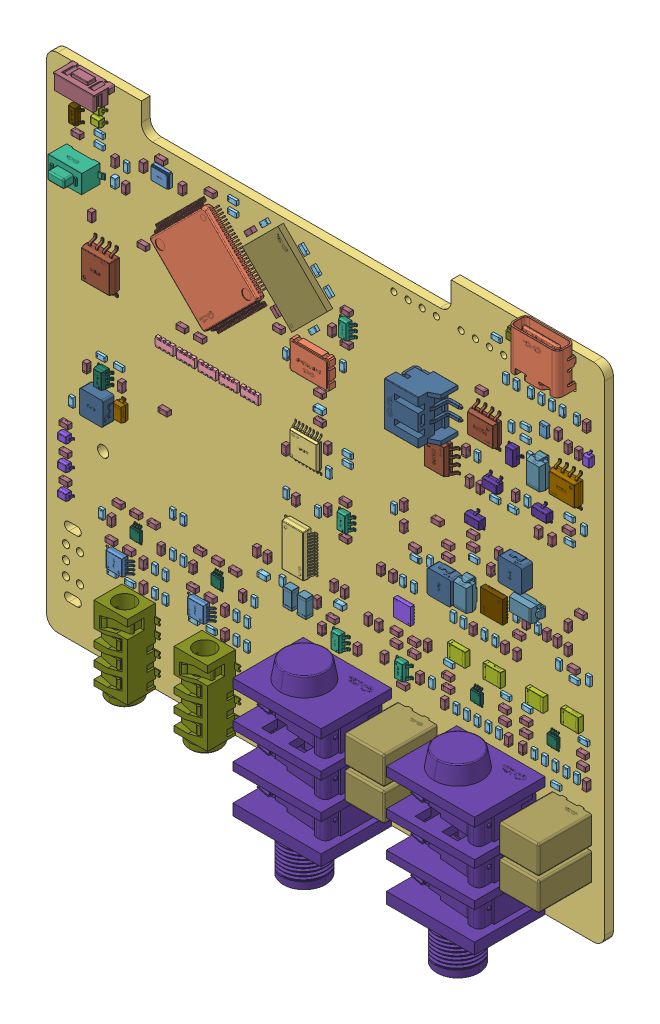
SolidWorks assembly 3D_board_2024-11-06, configuration 默认. Lengths in mm.
Overall size (99.97 100.01 16.2).
845 component instances, 39 part files, 0 mates.
Components (placement in the parent):
- 3D_board_2024-11-06.step-1: 3D_board_2024-11-06.step [默认] at origin size (99.97 100.01 16.2)
  - iqks-X1.step-1: iqks-X1.step [默认] at (20.955 -9.525 1.5862) x (-1 0 0) z (0 0 1) size (3.2 2.5 0.81)
    - OSC-SMD_4P-L3.2-W2.5-BL.step-1: OSC-SMD_4P-L3.2-W2.5-BL.step [默认] at origin size (3.2 2.5 0.81)
      - SOLID.step-1: SOLID.step [默认] at origin size (3.2 2.5 0.81)
  - iqks-X2.step-1: iqks-X2.step [默认] at (48.2601 -24.765 1.5862) x (-1 0 0) z (0 0 1) size (7 5 1.32)
    - OSC-SMD_4P-L7.0-W5.0-BL.step-1: OSC-SMD_4P-L7.0-W5.0-BL.step [默认] at origin size (7 5 1.32)
      - COMPOUND.step-1: COMPOUND.step [默认] at origin size (7 5 1.32)
  - iqks-U22.step-1: iqks-U22.step [默认] at (45.7201 -54.6101 1.5862) x (-1 0 0) z (0 0 1) size (5.89 7.71 1.66)
    - SSOP-28_L10.2-W5.3-P0.65-LS7.8-BL.step-1: SSOP-28_L10.2-W5.3-P0.65-LS7.8-BL.step [默认] at origin size (5.89 7.71 1.66)
      - SOLID-0.step-1: SOLID-0.step [默认] at origin size (5.89 7.71 1.66)
  - iqks-RN4.step-1: iqks-RN4.step [默认] at (33.0201 -35.5601 1.5862) x (-1 0 0) z (0 0 1) size (3.2 1.6 0.5)
    - RES-ARRAY-SMD_0603-8P-L3.2-W1.6-BL.step-1: RES-ARRAY-SMD_0603-8P-L3.2-W1.6-BL.step [默认] at origin size (3.2 1.6 0.5)
      - COMPOUND-1.step-1: COMPOUND-1.step [默认] at origin size (3.2 1.6 0.5)
  - iqks-RN3.step-1: iqks-RN3.step [默认] at (29.2101 -35.5601 1.5862) x (-1 0 0) z (0 0 1) size (3.2 1.6 0.5)
    - RES-ARRAY-SMD_0603-8P-L3.2-W1.6-BL.step-1: RES-ARRAY-SMD_0603-8P-L3.2-W1.6-BL.step [默认] at origin size (3.2 1.6 0.5)
      - COMPOUND-1.step-1: COMPOUND-1.step [默认] at origin size (3.2 1.6 0.5)
  - iqks-RN2.step-1: iqks-RN2.step [默认] at (25.4001 -35.5601 1.5862) x (-1 0 0) z (0 0 1) size (3.2 1.6 0.5)
    - RES-ARRAY-SMD_0603-8P-L3.2-W1.6-BL.step-1: RES-ARRAY-SMD_0603-8P-L3.2-W1.6-BL.step [默认] at origin size (3.2 1.6 0.5)
      - COMPOUND-1.step-1: COMPOUND-1.step [默认] at origin size (3.2 1.6 0.5)
  - iqks-RN1.step-1: iqks-RN1.step [默认] at (21.59 -35.5601 1.5862) x (-1 0 0) z (0 0 1) size (3.2 1.6 0.5)
    - RES-ARRAY-SMD_0603-8P-L3.2-W1.6-BL.step-1: RES-ARRAY-SMD_0603-8P-L3.2-W1.6-BL.step [默认] at origin size (3.2 1.6 0.5)
      - COMPOUND-1.step-1: COMPOUND-1.step [默认] at origin size (3.2 1.6 0.5)
  - iqks-RN5.step-1: iqks-RN5.step [默认] at (36.8301 -35.5601 1.5862) x (-1 0 0) z (0 0 1) size (3.2 1.6 0.5)
    - RES-ARRAY-SMD_0603-8P-L3.2-W1.6-BL.step-1: RES-ARRAY-SMD_0603-8P-L3.2-W1.6-BL.step [默认] at origin size (3.2 1.6 0.5)
      - COMPOUND-1.step-1: COMPOUND-1.step [默认] at origin size (3.2 1.6 0.5)
  - iqks-R53.step-1: iqks-R53.step [默认] at (90.8052 -10.16 1.5862) x (0 1 0) z (0 0 1) size (1.62 0.81 0.45)
    - R0603.step-1: R0603.step [默认] at origin size (1.62 0.81 0.45)
      - COMPOUND-2.step-1: COMPOUND-2.step [默认] at origin size (1.62 0.81 0.45)
  - iqks-R52.step-1: iqks-R52.step [默认] at (88.9002 -10.16 1.5862) x (0 1 0) z (0 0 1) size (1.62 0.81 0.45)
    - R0603.step-1: R0603.step [默认] at origin size (1.62 0.81 0.45)
      - COMPOUND-2.step-1: COMPOUND-2.step [默认] at origin size (1.62 0.81 0.45)
  - iqks-R7.step-1: iqks-R7.step [默认] at (72.3901 -59.4601 1.5862) size (1.62 0.81 0.45)
    - R0603.step-1: R0603.step [默认] at origin size (1.62 0.81 0.45)
      - COMPOUND-2.step-1: COMPOUND-2.step [默认] at origin size (1.62 0.81 0.45)
  - iqks-R14.step-1: iqks-R14.step [默认] at (82.5502 -59.4601 1.5862) x (-1 0 0) z (0 0 1) size (1.62 0.81 0.45)
    - R0603.step-1: R0603.step [默认] at origin size (1.62 0.81 0.45)
      - COMPOUND-2.step-1: COMPOUND-2.step [默认] at origin size (1.62 0.81 0.45)
  - iqks-R69.step-1: iqks-R69.step [默认] at (50.8001 -40.6401 1.5862) x (0 -1 0) z (0 0 1) size (1.62 0.81 0.45)
    - R0603.step-1: R0603.step [默认] at origin size (1.62 0.81 0.45)
      - COMPOUND-2.step-1: COMPOUND-2.step [默认] at origin size (1.62 0.81 0.45)
  - iqks-R55.step-1: iqks-R55.step [默认] at (84.4552 -10.16 1.5862) x (0 1 0) z (0 0 1) size (1.62 0.81 0.45)
    - R0603.step-1: R0603.step [默认] at origin size (1.62 0.81 0.45)
      - COMPOUND-2.step-1: COMPOUND-2.step [默认] at origin size (1.62 0.81 0.45)
  - iqks-R59.step-1: iqks-R59.step [默认] at (53.3401 -22.86 1.5862) x (0 1 0) z (0 0 1) size (1.62 0.81 0.45)
    - R0603.step-1: R0603.step [默认] at origin size (1.62 0.81 0.45)
      - COMPOUND-2.step-1: COMPOUND-2.step [默认] at origin size (1.62 0.81 0.45)
  - iqks-R62.step-1: iqks-R62.step [默认] at (48.1331 -19.8896 1.5862) x (0.707107 0.707107 0) z (0 0 1) size (1.62 0.81 0.45)
    - R0603.step-1: R0603.step [默认] at origin size (1.62 0.81 0.45)
      - COMPOUND-2.step-1: COMPOUND-2.step [默认] at origin size (1.62 0.81 0.45)
  - iqks-R63.step-1: iqks-R63.step [默认] at (50.8248 -12.6064 1.5862) x (0.707107 -0.707107 0) z (0 0 1) size (1.62 0.81 0.45)
    - R0603.step-1: R0603.step [默认] at origin size (1.62 0.81 0.45)
      - COMPOUND-2.step-1: COMPOUND-2.step [默认] at origin size (1.62 0.81 0.45)
  - iqks-R64.step-1: iqks-R64.step [默认] at (46.3551 -8.255 1.5862) x (-0.707107 0.707107 0) z (0 0 1) size (1.62 0.81 0.45)
    - R0603.step-1: R0603.step [默认] at origin size (1.62 0.81 0.45)
      - COMPOUND-2.step-1: COMPOUND-2.step [默认] at origin size (1.62 0.81 0.45)
  - iqks-R65.step-1: iqks-R65.step [默认] at (10.1012 -43.0318 1.5862) size (1.62 0.81 0.45)
    - R0603.step-1: R0603.step [默认] at origin size (1.62 0.81 0.45)
      - COMPOUND-2.step-1: COMPOUND-2.step [默认] at origin size (1.62 0.81 0.45)
  - iqks-R66.step-1: iqks-R66.step [默认] at (39.3701 -7.62 1.5862) x (0.707107 0.707107 0) z (0 0 1) size (1.62 0.81 0.45)
    - R0603.step-1: R0603.step [默认] at origin size (1.62 0.81 0.45)
      - COMPOUND-2.step-1: COMPOUND-2.step [默认] at origin size (1.62 0.81 0.45)
  - iqks-R67.step-1: iqks-R67.step [默认] at (48.5635 -10.414 1.5862) x (-0.707107 0.707107 0) z (0 0 1) size (1.62 0.81 0.45)
    - R0603.step-1: R0603.step [默认] at origin size (1.62 0.81 0.45)
      - COMPOUND-2.step-1: COMPOUND-2.step [默认] at origin size (1.62 0.81 0.45)
  - iqks-R74.step-1: iqks-R74.step [默认] at (82.5502 -10.16 1.5862) x (0 1 0) z (0 0 1) size (1.62 0.81 0.45)
    - R0603.step-1: R0603.step [默认] at origin size (1.62 0.81 0.45)
      - COMPOUND-2.step-1: COMPOUND-2.step [默认] at origin size (1.62 0.81 0.45)
  - iqks-R75.step-1: iqks-R75.step [默认] at (14.605 -11.303 1.5862) x (0 -1 0) z (0 0 1) size (1.62 0.81 0.45)
    - R0603.step-1: R0603.step [默认] at origin size (1.62 0.81 0.45)
      - COMPOUND-2.step-1: COMPOUND-2.step [默认] at origin size (1.62 0.81 0.45)
  - iqks-R76.step-1: iqks-R76.step [默认] at (33.6551 -8.89 1.5862) size (1.62 0.81 0.45)
    - R0603.step-1: R0603.step [默认] at origin size (1.62 0.81 0.45)
      - COMPOUND-2.step-1: COMPOUND-2.step [默认] at origin size (1.62 0.81 0.45)
  - iqks-R100.step-1: iqks-R100.step [默认] at (43.1801 -47.6251 1.5862) x (0 -1 0) z (0 0 1) size (1.62 0.81 0.45)
    - R0603.step-1: R0603.step [默认] at origin size (1.62 0.81 0.45)
      - COMPOUND-2.step-1: COMPOUND-2.step [默认] at origin size (1.62 0.81 0.45)
  - iqks-R103.step-1: iqks-R103.step [默认] at (54.2291 -36.0681 1.5862) x (-1 0 0) z (0 0 1) size (1.62 0.81 0.45)
    - R0603.step-1: R0603.step [默认] at origin size (1.62 0.81 0.45)
      - COMPOUND-2.step-1: COMPOUND-2.step [默认] at origin size (1.62 0.81 0.45)
  - iqks-R104.step-1: iqks-R104.step [默认] at (54.2291 -37.5921 1.5862) x (-1 0 0) z (0 0 1) size (1.62 0.81 0.45)
    - R0603.step-1: R0603.step [默认] at origin size (1.62 0.81 0.45)
      - COMPOUND-2.step-1: COMPOUND-2.step [默认] at origin size (1.62 0.81 0.45)
  - iqks-R10.step-1: iqks-R10.step [默认] at (79.3752 -65.8101 1.5862) x (0 -1 0) z (0 0 1) size (1.62 0.81 0.45)
    - R0603.step-1: R0603.step [默认] at origin size (1.62 0.81 0.45)
      - COMPOUND-2.step-1: COMPOUND-2.step [默认] at origin size (1.62 0.81 0.45)
  - iqks-R11.step-1: iqks-R11.step [默认] at (75.5652 -65.8101 1.5862) x (0 -1 0) z (0 0 1) size (1.62 0.81 0.45)
    - R0603.step-1: R0603.step [默认] at origin size (1.62 0.81 0.45)
      - COMPOUND-2.step-1: COMPOUND-2.step [默认] at origin size (1.62 0.81 0.45)
  - iqks-R29.step-1: iqks-R29.step [默认] at (93.3452 -65.8101 1.5862) x (0 -1 0) z (0 0 1) size (1.62 0.81 0.45)
    - R0603.step-1: R0603.step [默认] at origin size (1.62 0.81 0.45)
      - COMPOUND-2.step-1: COMPOUND-2.step [默认] at origin size (1.62 0.81 0.45)
  - iqks-R30.step-1: iqks-R30.step [默认] at (89.5352 -65.8101 1.5862) x (0 -1 0) z (0 0 1) size (1.62 0.81 0.45)
    - R0603.step-1: R0603.step [默认] at origin size (1.62 0.81 0.45)
      - COMPOUND-2.step-1: COMPOUND-2.step [默认] at origin size (1.62 0.81 0.45)
  - iqks-R5.step-1: iqks-R5.step [默认] at (87.6302 -65.8101 1.5862) x (0 -1 0) z (0 0 1) size (1.62 0.81 0.45)
    - R0603.step-1: R0603.step [默认] at origin size (1.62 0.81 0.45)
      - COMPOUND-2.step-1: COMPOUND-2.step [默认] at origin size (1.62 0.81 0.45)
  - iqks-R12.step-1: iqks-R12.step [默认] at (81.2802 -65.8101 1.5862) x (0 -1 0) z (0 0 1) size (1.62 0.81 0.45)
    - R0603.step-1: R0603.step [默认] at origin size (1.62 0.81 0.45)
      - COMPOUND-2.step-1: COMPOUND-2.step [默认] at origin size (1.62 0.81 0.45)
  - iqks-R13.step-1: iqks-R13.step [默认] at (73.6601 -65.8101 1.5862) x (0 -1 0) z (0 0 1) size (1.62 0.81 0.45)
    - R0603.step-1: R0603.step [默认] at origin size (1.62 0.81 0.45)
      - COMPOUND-2.step-1: COMPOUND-2.step [默认] at origin size (1.62 0.81 0.45)
  - iqks-R31.step-1: iqks-R31.step [默认] at (95.2502 -65.8101 1.5862) x (0 -1 0) z (0 0 1) size (1.62 0.81 0.45)
    - R0603.step-1: R0603.step [默认] at origin size (1.62 0.81 0.45)
      - COMPOUND-2.step-1: COMPOUND-2.step [默认] at origin size (1.62 0.81 0.45)
  - iqks-R115.step-1: iqks-R115.step [默认] at (83.8202 -29.8451 1.5862) x (-1 0 0) z (0 0 1) size (1.62 0.81 0.45)
    - R0603.step-1: R0603.step [默认] at origin size (1.62 0.81 0.45)
      - COMPOUND-2.step-1: COMPOUND-2.step [默认] at origin size (1.62 0.81 0.45)
  - iqks-R122.step-1: iqks-R122.step [默认] at (76.8352 -41.0211 1.5862) x (-1 0 0) z (0 0 1) size (1.62 0.81 0.45)
    - R0603.step-1: R0603.step [默认] at origin size (1.62 0.81 0.45)
      - COMPOUND-2.step-1: COMPOUND-2.step [默认] at origin size (1.62 0.81 0.45)
  - iqks-R91.step-1: iqks-R91.step [默认] at (42.5451 -61.5951 1.5862) x (0 -1 0) z (0 0 1) size (1.62 0.81 0.45)
    - R0603.step-1: R0603.step [默认] at origin size (1.62 0.81 0.45)
      - COMPOUND-2.step-1: COMPOUND-2.step [默认] at origin size (1.62 0.81 0.45)
  - iqks-R92.step-1: iqks-R92.step [默认] at (48.8951 -47.6251 1.5862) x (0 -1 0) z (0 0 1) size (1.62 0.81 0.45)
    - R0603.step-1: R0603.step [默认] at origin size (1.62 0.81 0.45)
      - COMPOUND-2.step-1: COMPOUND-2.step [默认] at origin size (1.62 0.81 0.45)
  - iqks-R111.step-1: iqks-R111.step [默认] at (24.765 -60.9601 1.5862) x (0 1 0) z (0 0 1) size (1.62 0.81 0.45)
    - R0603.step-1: R0603.step [默认] at origin size (1.62 0.81 0.45)
      - COMPOUND-2.step-1: COMPOUND-2.step [默认] at origin size (1.62 0.81 0.45)
  - iqks-R112.step-1: iqks-R112.step [默认] at (86.3602 -27.3051 1.5862) x (0 -1 0) z (0 0 1) size (1.62 0.81 0.45)
    - R0603.step-1: R0603.step [默认] at origin size (1.62 0.81 0.45)
      - COMPOUND-2.step-1: COMPOUND-2.step [默认] at origin size (1.62 0.81 0.45)
  - iqks-R128.step-1: iqks-R128.step [默认] at (73.1521 -51.8161 1.5862) x (0 -1 0) z (0 0 1) size (1.62 0.81 0.45)
    - R0603.step-1: R0603.step [默认] at origin size (1.62 0.81 0.45)
      - COMPOUND-2.step-1: COMPOUND-2.step [默认] at origin size (1.62 0.81 0.45)
  - iqks-R113.step-1: iqks-R113.step [默认] at (77.4702 -24.765 1.5862) x (0 1 0) z (0 0 1) size (1.62 0.81 0.45)
    - R0603.step-1: R0603.step [默认] at origin size (1.62 0.81 0.45)
      - COMPOUND-2.step-1: COMPOUND-2.step [默认] at origin size (1.62 0.81 0.45)
  - iqks-R6.step-1: iqks-R6.step [默认] at (86.3602 -59.4601 1.5862) size (1.62 0.81 0.45)
    - R0603.step-1: R0603.step [默认] at origin size (1.62 0.81 0.45)
      - COMPOUND-2.step-1: COMPOUND-2.step [默认] at origin size (1.62 0.81 0.45)
  - iqks-R32.step-1: iqks-R32.step [默认] at (96.5202 -59.4601 1.5862) x (-1 0 0) z (0 0 1) size (1.62 0.81 0.45)
    - R0603.step-1: R0603.step [默认] at origin size (1.62 0.81 0.45)
      - COMPOUND-2.step-1: COMPOUND-2.step [默认] at origin size (1.62 0.81 0.45)
  - iqks-R9.step-1: iqks-R9.step [默认] at (91.4402 -65.8101 1.5862) x (0 1 0) z (0 0 1) size (1.62 0.81 0.45)
    - R0603.step-1: R0603.step [默认] at origin size (1.62 0.81 0.45)
      - COMPOUND-2.step-1: COMPOUND-2.step [默认] at origin size (1.62 0.81 0.45)
  - iqks-R16.step-1: iqks-R16.step [默认] at (77.4702 -65.8101 1.5862) x (0 1 0) z (0 0 1) size (1.62 0.81 0.45)
    - R0603.step-1: R0603.step [默认] at origin size (1.62 0.81 0.45)
      - COMPOUND-2.step-1: COMPOUND-2.step [默认] at origin size (1.62 0.81 0.45)
  - iqks-R48.step-1: iqks-R48.step [默认] at (86.9952 -10.16 1.5862) x (0 1 0) z (0 0 1) size (1.62 0.81 0.45)
    - R0603.step-1: R0603.step [默认] at origin size (1.62 0.81 0.45)
      - COMPOUND-2.step-1: COMPOUND-2.step [默认] at origin size (1.62 0.81 0.45)
  - iqks-R50.step-1: iqks-R50.step [默认] at (92.7102 -10.16 1.5862) x (0 1 0) z (0 0 1) size (1.62 0.81 0.45)
    - R0603.step-1: R0603.step [默认] at origin size (1.62 0.81 0.45)
      - COMPOUND-2.step-1: COMPOUND-2.step [默认] at origin size (1.62 0.81 0.45)
  - iqks-R114.step-1: iqks-R114.step [默认] at (80.6452 -29.8451 1.5862) x (-1 0 0) z (0 0 1) size (1.62 0.81 0.45)
    - R0603.step-1: R0603.step [默认] at origin size (1.62 0.81 0.45)
      - COMPOUND-2.step-1: COMPOUND-2.step [默认] at origin size (1.62 0.81 0.45)
  - iqks-R21.step-1: iqks-R21.step [默认] at (19.685 -71.1201 1.5862) x (0 -1 0) z (0 0 1) size (1.62 0.81 0.45)
    - R0603.step-1: R0603.step [默认] at origin size (1.62 0.81 0.45)
      - COMPOUND-2.step-1: COMPOUND-2.step [默认] at origin size (1.62 0.81 0.45)
  - iqks-R22.step-1: iqks-R22.step [默认] at (19.685 -74.9301 1.5862) x (0 -1 0) z (0 0 1) size (1.62 0.81 0.45)
    - R0603.step-1: R0603.step [默认] at origin size (1.62 0.81 0.45)
      - COMPOUND-2.step-1: COMPOUND-2.step [默认] at origin size (1.62 0.81 0.45)
  - iqks-R25.step-1: iqks-R25.step [默认] at (34.2901 -71.1201 1.5862) x (0 -1 0) z (0 0 1) size (1.62 0.81 0.45)
    - R0603.step-1: R0603.step [默认] at origin size (1.62 0.81 0.45)
      - COMPOUND-2.step-1: COMPOUND-2.step [默认] at origin size (1.62 0.81 0.45)
  - iqks-R26.step-1: iqks-R26.step [默认] at (34.2901 -74.9301 1.5862) x (0 -1 0) z (0 0 1) size (1.62 0.81 0.45)
    - R0603.step-1: R0603.step [默认] at origin size (1.62 0.81 0.45)
      - COMPOUND-2.step-1: COMPOUND-2.step [默认] at origin size (1.62 0.81 0.45)
  - iqks-R116.step-1: iqks-R116.step [默认] at (96.5202 -26.6701 1.5862) x (0 1 0) z (0 0 1) size (1.62 0.81 0.45)
    - R0603.step-1: R0603.step [默认] at origin size (1.62 0.81 0.45)
      - COMPOUND-2.step-1: COMPOUND-2.step [默认] at origin size (1.62 0.81 0.45)
  - iqks-R2.step-1: iqks-R2.step [默认] at (21.59 -71.1201 1.5862) x (0 -1 0) z (0 0 1) size (1.62 0.81 0.45)
    - R0603.step-1: R0603.step [默认] at origin size (1.62 0.81 0.45)
      - COMPOUND-2.step-1: COMPOUND-2.step [默认] at origin size (1.62 0.81 0.45)
  - iqks-R4.step-1: iqks-R4.step [默认] at (21.59 -74.9301 1.5862) x (0 1 0) z (0 0 1) size (1.62 0.81 0.45)
    - R0603.step-1: R0603.step [默认] at origin size (1.62 0.81 0.45)
      - COMPOUND-2.step-1: COMPOUND-2.step [默认] at origin size (1.62 0.81 0.45)
  - iqks-R19.step-1: iqks-R19.step [默认] at (36.1951 -71.1201 1.5862) x (0 -1 0) z (0 0 1) size (1.62 0.81 0.45)
    - R0603.step-1: R0603.step [默认] at origin size (1.62 0.81 0.45)
      - COMPOUND-2.step-1: COMPOUND-2.step [默认] at origin size (1.62 0.81 0.45)
  - iqks-R20.step-1: iqks-R20.step [默认] at (36.1951 -74.9301 1.5862) x (0 1 0) z (0 0 1) size (1.62 0.81 0.45)
    - R0603.step-1: R0603.step [默认] at origin size (1.62 0.81 0.45)
      - COMPOUND-2.step-1: COMPOUND-2.step [默认] at origin size (1.62 0.81 0.45)
  - iqks-R110.step-1: iqks-R110.step [默认] at (22.86 -60.9601 1.5862) x (0 1 0) z (0 0 1) size (1.62 0.81 0.45)
    - R0603.step-1: R0603.step [默认] at origin size (1.62 0.81 0.45)
      - COMPOUND-2.step-1: COMPOUND-2.step [默认] at origin size (1.62 0.81 0.45)
  - iqks-R117.step-1: iqks-R117.step [默认] at (93.9802 -26.0351 1.5862) x (-1 0 0) z (0 0 1) size (1.62 0.81 0.45)
    - R0603.step-1: R0603.step [默认] at origin size (1.62 0.81 0.45)
      - COMPOUND-2.step-1: COMPOUND-2.step [默认] at origin size (1.62 0.81 0.45)
  - iqks-R1.step-1: iqks-R1.step [默认] at (10.16 -67.3101 1.5862) x (0 -1 0) z (0 0 1) size (1.62 0.81 0.45)
    - R0603.step-1: R0603.step [默认] at origin size (1.62 0.81 0.45)
      - COMPOUND-2.step-1: COMPOUND-2.step [默认] at origin size (1.62 0.81 0.45)
  - iqks-R3.step-1: iqks-R3.step [默认] at (22.86 -67.3101 1.5862) x (0 -1 0) z (0 0 1) size (1.62 0.81 0.45)
    - R0603.step-1: R0603.step [默认] at origin size (1.62 0.81 0.45)
      - COMPOUND-2.step-1: COMPOUND-2.step [默认] at origin size (1.62 0.81 0.45)
  - iqks-R17.step-1: iqks-R17.step [默认] at (37.4651 -67.3101 1.5862) x (0 -1 0) z (0 0 1) size (1.62 0.81 0.45)
    - R0603.step-1: R0603.step [默认] at origin size (1.62 0.81 0.45)
      - COMPOUND-2.step-1: COMPOUND-2.step [默认] at origin size (1.62 0.81 0.45)
  - iqks-R18.step-1: iqks-R18.step [默认] at (24.765 -67.3101 1.5862) x (0 -1 0) z (0 0 1) size (1.62 0.81 0.45)
    - R0603.step-1: R0603.step [默认] at origin size (1.62 0.81 0.45)
      - COMPOUND-2.step-1: COMPOUND-2.step [默认] at origin size (1.62 0.81 0.45)
  - iqks-R121.step-1: iqks-R121.step [默认] at (86.8682 -20.32 1.5862) x (0 1 0) z (0 0 1) size (1.62 0.81 0.45)
    - R0603.step-1: R0603.step [默认] at origin size (1.62 0.81 0.45)
      - COMPOUND-2.step-1: COMPOUND-2.step [默认] at origin size (1.62 0.81 0.45)
  - iqks-R120.step-1: iqks-R120.step [默认] at (86.1062 -17.78 1.5862) x (-1 0 0) z (0 0 1) size (1.62 0.81 0.45)
    - R0603.step-1: R0603.step [默认] at origin size (1.62 0.81 0.45)
      - COMPOUND-2.step-1: COMPOUND-2.step [默认] at origin size (1.62 0.81 0.45)
  - iqks-R118.step-1: iqks-R118.step [默认] at (80.8992 -4.699 1.5862) x (-1 0 0) z (0 0 1) size (1.62 0.81 0.45)
    - R0603.step-1: R0603.step [默认] at origin size (1.62 0.81 0.45)
      - COMPOUND-2.step-1: COMPOUND-2.step [默认] at origin size (1.62 0.81 0.45)
  - iqks-R119.step-1: iqks-R119.step [默认] at (83.5662 -17.145 1.5862) x (0 -1 0) z (0 0 1) size (1.62 0.81 0.45)
    - R0603.step-1: R0603.step [默认] at origin size (1.62 0.81 0.45)
      - COMPOUND-2.step-1: COMPOUND-2.step [默认] at origin size (1.62 0.81 0.45)
  - iqks-R23.step-1: iqks-R23.step [默认] at (15.24 -75.5652 1.5862) x (-1 0 0) z (0 0 1) size (1.62 0.81 0.45)
    - R0603.step-1: R0603.step [默认] at origin size (1.62 0.81 0.45)
      - COMPOUND-2.step-1: COMPOUND-2.step [默认] at origin size (1.62 0.81 0.45)
  - iqks-R24.step-1: iqks-R24.step [默认] at (12.065 -75.5652 1.5862) x (-1 0 0) z (0 0 1) size (1.62 0.81 0.45)
    - R0603.step-1: R0603.step [默认] at origin size (1.62 0.81 0.45)
      - COMPOUND-2.step-1: COMPOUND-2.step [默认] at origin size (1.62 0.81 0.45)
  - iqks-R27.step-1: iqks-R27.step [默认] at (29.8451 -75.5652 1.5862) x (-1 0 0) z (0 0 1) size (1.62 0.81 0.45)
    - R0603.step-1: R0603.step [默认] at origin size (1.62 0.81 0.45)
      - COMPOUND-2.step-1: COMPOUND-2.step [默认] at origin size (1.62 0.81 0.45)
  - iqks-R28.step-1: iqks-R28.step [默认] at (26.6701 -75.5652 1.5862) x (-1 0 0) z (0 0 1) size (1.62 0.81 0.45)
    - R0603.step-1: R0603.step [默认] at origin size (1.62 0.81 0.45)
      - COMPOUND-2.step-1: COMPOUND-2.step [默认] at origin size (1.62 0.81 0.45)
  - iqks-R123.step-1: iqks-R123.step [默认] at (74.9301 -51.8161 1.5862) x (0 -1 0) z (0 0 1) size (1.62 0.81 0.45)
    - R0603.step-1: R0603.step [默认] at origin size (1.62 0.81 0.45)
      - COMPOUND-2.step-1: COMPOUND-2.step [默认] at origin size (1.62 0.81 0.45)
  - iqks-R49.step-1: iqks-R49.step [默认] at (95.2502 -10.16 1.5862) x (0 1 0) z (0 0 1) size (1.62 0.81 0.45)
    - R0603.step-1: R0603.step [默认] at origin size (1.62 0.81 0.45)
      - COMPOUND-2.step-1: COMPOUND-2.step [默认] at origin size (1.62 0.81 0.45)
  - iqks-R124.step-1: iqks-R124.step [默认] at (84.4552 -46.1011 1.5862) x (0 1 0) z (0 0 1) size (1.62 0.81 0.45)
    - R0603.step-1: R0603.step [默认] at origin size (1.62 0.81 0.45)
      - COMPOUND-2.step-1: COMPOUND-2.step [默认] at origin size (1.62 0.81 0.45)
  - iqks-R125.step-1: iqks-R125.step [默认] at (88.2652 -46.1011 1.5862) x (0 1 0) z (0 0 1) size (1.62 0.81 0.45)
    - R0603.step-1: R0603.step [默认] at origin size (1.62 0.81 0.45)
      - COMPOUND-2.step-1: COMPOUND-2.step [默认] at origin size (1.62 0.81 0.45)
  - iqks-R126.step-1: iqks-R126.step [默认] at (80.6452 -51.8161 1.5862) x (0 -1 0) z (0 0 1) size (1.62 0.81 0.45)
    - R0603.step-1: R0603.step [默认] at origin size (1.62 0.81 0.45)
      - COMPOUND-2.step-1: COMPOUND-2.step [默认] at origin size (1.62 0.81 0.45)
  - iqks-R127.step-1: iqks-R127.step [默认] at (78.7402 -51.8161 1.5862) x (0 1 0) z (0 0 1) size (1.62 0.81 0.45)
    - R0603.step-1: R0603.step [默认] at origin size (1.62 0.81 0.45)
      - COMPOUND-2.step-1: COMPOUND-2.step [默认] at origin size (1.62 0.81 0.45)
  - iqks-R129.step-1: iqks-R129.step [默认] at (68.9593 -45.3937 1.5862) x (0 -1 0) z (0 0 1) size (1.62 0.81 0.45)
    - R0603.step-1: R0603.step [默认] at origin size (1.62 0.81 0.45)
      - COMPOUND-2.step-1: COMPOUND-2.step [默认] at origin size (1.62 0.81 0.45)
  - iqks-R131.step-1: iqks-R131.step [默认] at (97.4092 -49.5301 1.5862) x (0 -1 0) z (0 0 1) size (1.62 0.81 0.45)
    - R0603.step-1: R0603.step [默认] at origin size (1.62 0.81 0.45)
      - COMPOUND-2.step-1: COMPOUND-2.step [默认] at origin size (1.62 0.81 0.45)
  - iqks-R132.step-1: iqks-R132.step [默认] at (94.8692 -50.8001 1.5862) x (-1 0 0) z (0 0 1) size (1.62 0.81 0.45)
    - R0603.step-1: R0603.step [默认] at origin size (1.62 0.81 0.45)
      - COMPOUND-2.step-1: COMPOUND-2.step [默认] at origin size (1.62 0.81 0.45)
  - iqks-R133.step-1: iqks-R133.step [默认] at (66.4193 -46.1557 1.5862) x (-1 0 0) z (0 0 1) size (1.62 0.81 0.45)
    - R0603.step-1: R0603.step [默认] at origin size (1.62 0.81 0.45)
      - COMPOUND-2.step-1: COMPOUND-2.step [默认] at origin size (1.62 0.81 0.45)
  - iqks-JP1.step-1: iqks-JP1.step [默认] at (93.9802 -29.8451 1.5862) x (-1 0 0) z (0 0 1) size (1.62 0.81 0.45)
    - R0603.step-1: R0603.step [默认] at origin size (1.62 0.81 0.45)
      - COMPOUND-2.step-1: COMPOUND-2.step [默认] at origin size (1.62 0.81 0.45)
  - iqks-JP2.step-1: iqks-JP2.step [默认] at (86.1062 -15.875 1.5862) x (-1 0 0) z (0 0 1) size (1.62 0.81 0.45)
    - R0603.step-1: R0603.step [默认] at origin size (1.62 0.81 0.45)
      - COMPOUND-2.step-1: COMPOUND-2.step [默认] at origin size (1.62 0.81 0.45)
  - iqks-JP4.step-1: iqks-JP4.step [默认] at (33.6551 -6.985 1.5862) size (1.62 0.81 0.45)
    - R0603.step-1: R0603.step [默认] at origin size (1.62 0.81 0.45)
      - COMPOUND-2.step-1: COMPOUND-2.step [默认] at origin size (1.62 0.81 0.45)
  - iqks-JP5.step-1: iqks-JP5.step [默认] at (92.0752 -49.7841 1.5862) x (0 -1 0) z (0 0 1) size (1.62 0.81 0.45)
    - R0603.step-1: R0603.step [默认] at origin size (1.62 0.81 0.45)
      - COMPOUND-2.step-1: COMPOUND-2.step [默认] at origin size (1.62 0.81 0.45)
  - iqks-JP6.step-1: iqks-JP6.step [默认] at (62.5179 -40.2999 1.5862) x (0 -1 0) z (0 0 1) size (1.62 0.81 0.45)
    - R0603.step-1: R0603.step [默认] at origin size (1.62 0.81 0.45)
      - COMPOUND-2.step-1: COMPOUND-2.step [默认] at origin size (1.62 0.81 0.45)
  - iqks-R101.step-1: iqks-R101.step [默认] at (64.1351 -50.8001 1.5862) x (0 1 0) z (0 0 1) size (1.62 0.81 0.45)
    - R0603.step-1: R0603.step [默认] at origin size (1.62 0.81 0.45)
      - COMPOUND-2.step-1: COMPOUND-2.step [默认] at origin size (1.62 0.81 0.45)
  - iqks-R102.step-1: iqks-R102.step [默认] at (66.0401 -50.8001 1.5862) x (0 1 0) z (0 0 1) size (1.62 0.81 0.45)
    - R0603.step-1: R0603.step [默认] at origin size (1.62 0.81 0.45)
      - COMPOUND-2.step-1: COMPOUND-2.step [默认] at origin size (1.62 0.81 0.45)
  - iqks-R109.step-1: iqks-R109.step [默认] at (43.1801 -26.0351 1.5862) x (0 1 0) z (0 0 1) size (1.62 0.81 0.45)
    - R0603.step-1: R0603.step [默认] at origin size (1.62 0.81 0.45)
      - COMPOUND-2.step-1: COMPOUND-2.step [默认] at origin size (1.62 0.81 0.45)
  - iqks-R134.step-1: iqks-R134.step [默认] at (80.0102 -77.9782 0) x (0 -1 0) z (0 0 -1) size (1.62 0.81 0.45)
    - R0603.step-1: R0603.step [默认] at origin size (1.62 0.81 0.45)
      - COMPOUND-2.step-1: COMPOUND-2.step [默认] at origin size (1.62 0.81 0.45)
  - iqks-R135.step-1: iqks-R135.step [默认] at (51.5621 -77.8512 0) x (0 -1 0) z (0 0 -1) size (1.62 0.81 0.45)
    - R0603.step-1: R0603.step [默认] at origin size (1.62 0.81 0.45)
      - COMPOUND-2.step-1: COMPOUND-2.step [默认] at origin size (1.62 0.81 0.45)
  - iqks-R138.step-1: iqks-R138.step [默认] at (9.779 -8.636 1.5862) x (-1 0 0) z (0 0 1) size (1.62 0.81 0.45)
    - R0603.step-1: R0603.step [默认] at origin size (1.62 0.81 0.45)
      - COMPOUND-2.step-1: COMPOUND-2.step [默认] at origin size (1.62 0.81 0.45)
  - iqks-R139.step-1: iqks-R139.step [默认] at (9.779 -10.414 1.5862) size (1.62 0.81 0.45)
    - R0603.step-1: R0603.step [默认] at origin size (1.62 0.81 0.45)
      - COMPOUND-2.step-1: COMPOUND-2.step [默认] at origin size (1.62 0.81 0.45)
  - iqks-R8.step-1: iqks-R8.step [默认] at (71.3741 -82.0822 1.5862) x (-1 0 0) z (0 0 1) size (1.62 0.81 0.45)
    - R0603.step-1: R0603.step [默认] at origin size (1.62 0.81 0.45)
      - COMPOUND-2.step-1: COMPOUND-2.step [默认] at origin size (1.62 0.81 0.45)
  - iqks-R15.step-1: iqks-R15.step [默认] at (64.0081 -82.0822 1.5862) size (1.62 0.81 0.45)
    - R0603.step-1: R0603.step [默认] at origin size (1.62 0.81 0.45)
      - COMPOUND-2.step-1: COMPOUND-2.step [默认] at origin size (1.62 0.81 0.45)
  - iqks-J8.step-1: iqks-J8.step [默认] at (4.826 -52.5781 1.5862) x (0 1 0) z (0 0 1) size (1.62 0.81 0.45)
    - R0603.step-1: R0603.step [默认] at origin size (1.62 0.81 0.45)
      - COMPOUND-2.step-1: COMPOUND-2.step [默认] at origin size (1.62 0.81 0.45)
  - iqks-J9.step-1: iqks-J9.step [默认] at (91.5672 -68.8341 1.5862) x (-1 0 0) z (0 0 1) size (1.62 0.81 0.45)
    - R0603.step-1: R0603.step [默认] at origin size (1.62 0.81 0.45)
      - COMPOUND-2.step-1: COMPOUND-2.step [默认] at origin size (1.62 0.81 0.45)
  - iqks-J10.step-1: iqks-J10.step [默认] at (69.3143 -63.9872 1.5862) x (0 -1 0) z (0 0 1) size (1.62 0.81 0.45)
    - R0603.step-1: R0603.step [默认] at origin size (1.62 0.81 0.45)
      - COMPOUND-2.step-1: COMPOUND-2.step [默认] at origin size (1.62 0.81 0.45)
  - iqks-R60.step-1: iqks-R60.step [默认] at (13.2762 -43.0318 1.5862) size (1.62 0.81 0.45)
    - R0603.step-1: R0603.step [默认] at origin size (1.62 0.81 0.45)
      - COMPOUND-2.step-1: COMPOUND-2.step [默认] at origin size (1.62 0.81 0.45)
  - iqks-SW3.step-1: iqks-SW3.step [默认] at (6.604 -14.986 1.5862) size (8 3.3 5)
    - SW-SMD_L6.0-W3.3-LS8.0.step-1: SW-SMD_L6.0-W3.3-LS8.0.step [默认] at origin size (8 3.3 5)
      - SOLID-3.step-1: SOLID-3.step [默认] at origin size (8 3.3 5)
  - iqks-C130.step-1: iqks-C130.step [默认] at (94.6152 -56.9201 1.5862) size (3.2 2.52 0.9)
    - C1210.step-1: C1210.step [默认] at origin size (3.2 2.52 0.9)
      - SOLID-4.step-1: SOLID-4.step [默认] at origin size (3.2 2.52 0.9)
  - iqks-C35.step-1: iqks-C35.step [默认] at (88.2652 -56.9201 1.5862) x (-1 0 0) z (0 0 1) size (3.2 2.52 0.9)
    - C1210.step-1: C1210.step [默认] at origin size (3.2 2.52 0.9)
      - SOLID-4.step-1: SOLID-4.step [默认] at origin size (3.2 2.52 0.9)
  - iqks-C34.step-1: iqks-C34.step [默认] at (80.6452 -56.9201 1.5862) size (3.2 2.52 0.9)
    - C1210.step-1: C1210.step [默认] at origin size (3.2 2.52 0.9)
      - SOLID-4.step-1: SOLID-4.step [默认] at origin size (3.2 2.52 0.9)
  - iqks-C131.step-1: iqks-C131.step [默认] at (74.2951 -56.9201 1.5862) x (-1 0 0) z (0 0 1) size (3.2 2.52 0.9)
    - C1210.step-1: C1210.step [默认] at origin size (3.2 2.52 0.9)
      - SOLID-4.step-1: SOLID-4.step [默认] at origin size (3.2 2.52 0.9)
  - iqks-D7.step-1: iqks-D7.step [默认] at (3.81 -62.8651 1.5862) size (2.5 1.3 1.1)
    - SOD-323_L1.7-W1.3-LS2.5-BI.step-1: SOD-323_L1.7-W1.3-LS2.5-BI.step [默认] at origin size (2.5 1.3 1.1)
      - COMPOUND-5.step-1: COMPOUND-5.step [默认] at origin size (2.5 1.3 1.1)
  - iqks-D6.step-1: iqks-D6.step [默认] at (3.81 -58.4201 1.5862) x (-1 0 0) z (0 0 1) size (2.5 1.3 1.1)
    - SOD-323_L1.7-W1.3-LS2.5-BI.step-1: SOD-323_L1.7-W1.3-LS2.5-BI.step [默认] at origin size (2.5 1.3 1.1)
      - COMPOUND-5.step-1: COMPOUND-5.step [默认] at origin size (2.5 1.3 1.1)
  - iqks-D8.step-1: iqks-D8.step [默认] at (97.6632 -15.113 1.5862) x (0 -1 0) z (0 0 1) size (2.5 1.3 1.1)
    - SOD-323_L1.7-W1.3-LS2.5-BI.step-1: SOD-323_L1.7-W1.3-LS2.5-BI.step [默认] at origin size (2.5 1.3 1.1)
      - COMPOUND-5.step-1: COMPOUND-5.step [默认] at origin size (2.5 1.3 1.1)
  - iqks-D5.step-1: iqks-D5.step [默认] at (3.81 -67.3101 1.5862) size (2.5 1.3 1.1)
    - SOD-323_L1.7-W1.3-LS2.5-BI.step-1: SOD-323_L1.7-W1.3-LS2.5-BI.step [默认] at origin size (2.5 1.3 1.1)
      - COMPOUND-5.step-1: COMPOUND-5.step [默认] at origin size (2.5 1.3 1.1)
  - iqks-D4.step-1: iqks-D4.step [默认] at (13.9112 -49.3818 1.5862) x (0 -1 0) z (0 0 1) size (3.68 1.6 1.22)
    - SOD-123_L2.8-W1.8-LS3.7-RD.step-1: SOD-123_L2.8-W1.8-LS3.7-RD.step [默认] at origin size (3.68 1.6 1.22)
      - SOLID-6.step-1: SOLID-6.step [默认] at origin size (3.68 1.6 1.22)
  - iqks-L2.step-1: iqks-L2.step [默认] at (85.0902 -38.4811 1.5862) x (0 1 0) z (0 0 1) size (4.4 4.2 2.1)
    - IND-SMD_L4.4-W4.2.step-1: IND-SMD_L4.4-W4.2.step [默认] at origin size (4.4 4.2 2.1)
      - SOLID-7.step-1: SOLID-7.step [默认] at origin size (4.4 4.2 2.1)
  - iqks-L3.step-1: iqks-L3.step [默认] at (72.3901 -46.7361 1.5862) x (0 1 0) z (0 0 1) size (4.4 4.2 2.1)
    - IND-SMD_L4.4-W4.2.step-1: IND-SMD_L4.4-W4.2.step [默认] at origin size (4.4 4.2 2.1)
      - SOLID-7.step-1: SOLID-7.step [默认] at origin size (4.4 4.2 2.1)
  - iqks-L7.step-1: iqks-L7.step [默认] at (10.1012 -50.0168 1.5862) size (4.4 4.2 2.1)
    - IND-SMD_L4.4-W4.2.step-1: IND-SMD_L4.4-W4.2.step [默认] at origin size (4.4 4.2 2.1)
      - SOLID-7.step-1: SOLID-7.step [默认] at origin size (4.4 4.2 2.1)
  - iqks-U20.step-1: iqks-U20.step [默认] at (10.795 -28.5751 1.5862) size (5.3 7.91 2.07)
    - SOIC-8_L5.3-W5.3-P1.27-LS8.0-BL.step-1: SOIC-8_L5.3-W5.3-P1.27-LS8.0-BL.step [默认] at origin size (5.3 7.91 2.07)
      - COMPOUND-8.step-1: COMPOUND-8.step [默认] at origin size (5.3 7.91 2.07)
  - iqks-C40.step-1: iqks-C40.step [默认] at (94.3612 -72.5251 1.5862) size (7.2 5 13.3)
    - CAP-TH_L7.2-W5.0-P5.00-D1.0.step-1: CAP-TH_L7.2-W5.0-P5.00-D1.0.step [默认] at origin size (7.2 5 13.3)
      - SOLID-9.step-1: SOLID-9.step [默认] at origin size (7.2 5 13.3)
  - iqks-C12.step-1: iqks-C12.step [默认] at (66.6751 -78.2402 1.5862) size (7.2 5 13.3)
    - CAP-TH_L7.2-W5.0-P5.00-D1.0.step-1: CAP-TH_L7.2-W5.0-P5.00-D1.0.step [默认] at origin size (7.2 5 13.3)
      - SOLID-9.step-1: SOLID-9.step [默认] at origin size (7.2 5 13.3)
  - iqks-C47.step-1: iqks-C47.step [默认] at (66.6751 -72.5251 1.5862) size (7.2 5 13.3)
    - CAP-TH_L7.2-W5.0-P5.00-D1.0.step-1: CAP-TH_L7.2-W5.0-P5.00-D1.0.step [默认] at origin size (7.2 5 13.3)
      - SOLID-9.step-1: SOLID-9.step [默认] at origin size (7.2 5 13.3)
  - iqks-C41.step-1: iqks-C41.step [默认] at (94.3612 -78.2402 1.5862) size (7.2 5 13.3)
    - CAP-TH_L7.2-W5.0-P5.00-D1.0.step-1: CAP-TH_L7.2-W5.0-P5.00-D1.0.step [默认] at origin size (7.2 5 13.3)
      - SOLID-9.step-1: SOLID-9.step [默认] at origin size (7.2 5 13.3)
  - iqks-C114.step-1: iqks-C114.step [默认] at (45.0851 -47.6251 1.5862) x (0 1 0) z (0 0 1) size (1.6 0.8 0.8)
    - C0603.step-1: C0603.step [默认] at origin size (1.6 0.8 0.8)
      - SOLID-10.step-1: SOLID-10.step [默认] at origin size (1.6 0.8 0.8)
  - iqks-C102.step-1: iqks-C102.step [默认] at (17.78 -21.844 1.5862) x (-1 0 0) z (0 0 1) size (1.6 0.8 0.8)
    - C0603.step-1: C0603.step [默认] at origin size (1.6 0.8 0.8)
      - SOLID-10.step-1: SOLID-10.step [默认] at origin size (1.6 0.8 0.8)
  - iqks-C101.step-1: iqks-C101.step [默认] at (8.5117 -21.8363 1.5862) x (0 1 0) z (0 0 1) size (1.6 0.8 0.8)
    - C0603.step-1: C0603.step [默认] at origin size (1.6 0.8 0.8)
      - SOLID-10.step-1: SOLID-10.step [默认] at origin size (1.6 0.8 0.8)
  - iqks-C100.step-1: iqks-C100.step [默认] at (21.59 -45.5931 1.5862) x (-1 0 0) z (0 0 1) size (1.6 0.8 0.8)
    - C0603.step-1: C0603.step [默认] at origin size (1.6 0.8 0.8)
      - SOLID-10.step-1: SOLID-10.step [默认] at origin size (1.6 0.8 0.8)
  - iqks-C93.step-1: iqks-C93.step [默认] at (13.9112 -45.5718 1.5862) x (0 1 0) z (0 0 1) size (1.6 0.8 0.8)
    - C0603.step-1: C0603.step [默认] at origin size (1.6 0.8 0.8)
      - SOLID-10.step-1: SOLID-10.step [默认] at origin size (1.6 0.8 0.8)
  - iqks-C92.step-1: iqks-C92.step [默认] at (50.8001 -36.765 1.5862) x (0 1 0) z (0 0 1) size (1.6 0.8 0.8)
    - C0603.step-1: C0603.step [默认] at origin size (1.6 0.8 0.8)
      - SOLID-10.step-1: SOLID-10.step [默认] at origin size (1.6 0.8 0.8)
  - iqks-C91.step-1: iqks-C91.step [默认] at (36.9571 -10.033 1.5862) x (-0.707107 -0.707107 0) z (0 0 1) size (1.6 0.8 0.8)
    - C0603.step-1: C0603.step [默认] at origin size (1.6 0.8 0.8)
      - SOLID-10.step-1: SOLID-10.step [默认] at origin size (1.6 0.8 0.8)
  - iqks-C90.step-1: iqks-C90.step [默认] at (43.3071 -40.6401 1.5862) x (0 1 0) z (0 0 1) size (1.6 0.8 0.8)
    - C0603.step-1: C0603.step [默认] at origin size (1.6 0.8 0.8)
      - SOLID-10.step-1: SOLID-10.step [默认] at origin size (1.6 0.8 0.8)
  - iqks-C89.step-1: iqks-C89.step [默认] at (7.62 -45.7201 1.5862) x (0 -1 0) z (0 0 1) size (1.6 0.8 0.8)
    - C0603.step-1: C0603.step [默认] at origin size (1.6 0.8 0.8)
      - SOLID-10.step-1: SOLID-10.step [默认] at origin size (1.6 0.8 0.8)
  - iqks-C87.step-1: iqks-C87.step [默认] at (49.4031 -28.9561 1.5862) x (-1 0 0) z (0 0 1) size (1.6 0.8 0.8)
    - C0603.step-1: C0603.step [默认] at origin size (1.6 0.8 0.8)
      - SOLID-10.step-1: SOLID-10.step [默认] at origin size (1.6 0.8 0.8)
  - iqks-C86.step-1: iqks-C86.step [默认] at (3.81 -60.9601 1.5862) x (-1 0 0) z (0 0 1) size (1.6 0.8 0.8)
    - C0603.step-1: C0603.step [默认] at origin size (1.6 0.8 0.8)
      - SOLID-10.step-1: SOLID-10.step [默认] at origin size (1.6 0.8 0.8)
  - iqks-C85.step-1: iqks-C85.step [默认] at (3.81 -65.4051 1.5862) x (-1 0 0) z (0 0 1) size (1.6 0.8 0.8)
    - C0603.step-1: C0603.step [默认] at origin size (1.6 0.8 0.8)
      - SOLID-10.step-1: SOLID-10.step [默认] at origin size (1.6 0.8 0.8)
  - iqks-C84.step-1: iqks-C84.step [默认] at (3.81 -56.5151 1.5862) size (1.6 0.8 0.8)
    - C0603.step-1: C0603.step [默认] at origin size (1.6 0.8 0.8)
      - SOLID-10.step-1: SOLID-10.step [默认] at origin size (1.6 0.8 0.8)
  - iqks-C82.step-1: iqks-C82.step [默认] at (42.0371 -22.606 1.5862) size (1.6 0.8 0.8)
    - C0603.step-1: C0603.step [默认] at origin size (1.6 0.8 0.8)
      - SOLID-10.step-1: SOLID-10.step [默认] at origin size (1.6 0.8 0.8)
  - iqks-C81.step-1: iqks-C81.step [默认] at (29.8451 -7.62 1.5862) x (-1 0 0) z (0 0 1) size (1.6 0.8 0.8)
    - C0603.step-1: C0603.step [默认] at origin size (1.6 0.8 0.8)
      - SOLID-10.step-1: SOLID-10.step [默认] at origin size (1.6 0.8 0.8)
  - iqks-C80.step-1: iqks-C80.step [默认] at (12.7 -11.303 1.5862) x (0 1 0) z (0 0 1) size (1.6 0.8 0.8)
    - C0603.step-1: C0603.step [默认] at origin size (1.6 0.8 0.8)
      - SOLID-10.step-1: SOLID-10.step [默认] at origin size (1.6 0.8 0.8)
  - iqks-C79.step-1: iqks-C79.step [默认] at (24.765 -9.525 1.5862) x (0 1 0) z (0 0 1) size (1.6 0.8 0.8)
    - C0603.step-1: C0603.step [默认] at origin size (1.6 0.8 0.8)
      - SOLID-10.step-1: SOLID-10.step [默认] at origin size (1.6 0.8 0.8)
  - iqks-C78.step-1: iqks-C78.step [默认] at (24.765 -31.1151 1.5862) x (-1 0 0) z (0 0 1) size (1.6 0.8 0.8)
    - C0603.step-1: C0603.step [默认] at origin size (1.6 0.8 0.8)
      - SOLID-10.step-1: SOLID-10.step [默认] at origin size (1.6 0.8 0.8)
  - iqks-C77.step-1: iqks-C77.step [默认] at (14.605 -14.478 1.5862) x (0 1 0) z (0 0 1) size (1.6 0.8 0.8)
    - C0603.step-1: C0603.step [默认] at origin size (1.6 0.8 0.8)
      - SOLID-10.step-1: SOLID-10.step [默认] at origin size (1.6 0.8 0.8)
  - iqks-C76.step-1: iqks-C76.step [默认] at (41.6561 -20.066 1.5862) x (0.707107 -0.707107 0) z (0 0 1) size (1.6 0.8 0.8)
    - C0603.step-1: C0603.step [默认] at origin size (1.6 0.8 0.8)
      - SOLID-10.step-1: SOLID-10.step [默认] at origin size (1.6 0.8 0.8)
  - iqks-C75.step-1: iqks-C75.step [默认] at (20.955 -6.985 1.5862) x (-1 0 0) z (0 0 1) size (1.6 0.8 0.8)
    - C0603.step-1: C0603.step [默认] at origin size (1.6 0.8 0.8)
      - SOLID-10.step-1: SOLID-10.step [默认] at origin size (1.6 0.8 0.8)
  - iqks-C73.step-1: iqks-C73.step [默认] at (27.9401 -31.1151 1.5862) size (1.6 0.8 0.8)
    - C0603.step-1: C0603.step [默认] at origin size (1.6 0.8 0.8)
      - SOLID-10.step-1: SOLID-10.step [默认] at origin size (1.6 0.8 0.8)
  - iqks-C71.step-1: iqks-C71.step [默认] at (17.78 -9.525 1.5862) x (0 1 0) z (0 0 1) size (1.6 0.8 0.8)
    - C0603.step-1: C0603.step [默认] at origin size (1.6 0.8 0.8)
      - SOLID-10.step-1: SOLID-10.step [默认] at origin size (1.6 0.8 0.8)
  - iqks-C69.step-1: iqks-C69.step [默认] at (97.1552 -10.16 1.5862) x (0 -1 0) z (0 0 1) size (1.6 0.8 0.8)
    - C0603.step-1: C0603.step [默认] at origin size (1.6 0.8 0.8)
      - SOLID-10.step-1: SOLID-10.step [默认] at origin size (1.6 0.8 0.8)
  - iqks-C8.step-1: iqks-C8.step [默认] at (86.3602 -63.2701 1.5862) size (1.6 0.8 0.8)
    - C0603.step-1: C0603.step [默认] at origin size (1.6 0.8 0.8)
      - SOLID-10.step-1: SOLID-10.step [默认] at origin size (1.6 0.8 0.8)
  - iqks-C6.step-1: iqks-C6.step [默认] at (96.5202 -61.3651 1.5862) x (-1 0 0) z (0 0 1) size (1.6 0.8 0.8)
    - C0603.step-1: C0603.step [默认] at origin size (1.6 0.8 0.8)
      - SOLID-10.step-1: SOLID-10.step [默认] at origin size (1.6 0.8 0.8)
  - iqks-C13.step-1: iqks-C13.step [默认] at (82.5502 -63.2701 1.5862) x (-1 0 0) z (0 0 1) size (1.6 0.8 0.8)
    - C0603.step-1: C0603.step [默认] at origin size (1.6 0.8 0.8)
      - SOLID-10.step-1: SOLID-10.step [默认] at origin size (1.6 0.8 0.8)
  - iqks-C11.step-1: iqks-C11.step [默认] at (72.3901 -63.2701 1.5862) size (1.6 0.8 0.8)
    - C0603.step-1: C0603.step [默认] at origin size (1.6 0.8 0.8)
      - SOLID-10.step-1: SOLID-10.step [默认] at origin size (1.6 0.8 0.8)
  - iqks-C7.step-1: iqks-C7.step [默认] at (86.3602 -61.3651 1.5862) x (-1 0 0) z (0 0 1) size (1.6 0.8 0.8)
    - C0603.step-1: C0603.step [默认] at origin size (1.6 0.8 0.8)
      - SOLID-10.step-1: SOLID-10.step [默认] at origin size (1.6 0.8 0.8)
  - iqks-C10.step-1: iqks-C10.step [默认] at (72.3901 -61.3651 1.5862) x (-1 0 0) z (0 0 1) size (1.6 0.8 0.8)
    - C0603.step-1: C0603.step [默认] at origin size (1.6 0.8 0.8)
      - SOLID-10.step-1: SOLID-10.step [默认] at origin size (1.6 0.8 0.8)
  - iqks-C14.step-1: iqks-C14.step [默认] at (82.5502 -61.3651 1.5862) x (-1 0 0) z (0 0 1) size (1.6 0.8 0.8)
    - C0603.step-1: C0603.step [默认] at origin size (1.6 0.8 0.8)
      - SOLID-10.step-1: SOLID-10.step [默认] at origin size (1.6 0.8 0.8)
  - iqks-C37.step-1: iqks-C37.step [默认] at (96.5202 -63.2701 1.5862) x (-1 0 0) z (0 0 1) size (1.6 0.8 0.8)
    - C0603.step-1: C0603.step [默认] at origin size (1.6 0.8 0.8)
      - SOLID-10.step-1: SOLID-10.step [默认] at origin size (1.6 0.8 0.8)
  - iqks-C45.step-1: iqks-C45.step [默认] at (95.7582 -15.113 1.5862) x (0 -1 0) z (0 0 1) size (1.6 0.8 0.8)
    - C0603.step-1: C0603.step [默认] at origin size (1.6 0.8 0.8)
      - SOLID-10.step-1: SOLID-10.step [默认] at origin size (1.6 0.8 0.8)
  - iqks-C48.step-1: iqks-C48.step [默认] at (88.5625 -30.9354 1.5862) x (0 1 0) z (0 0 1) size (1.6 0.8 0.8)
    - C0603.step-1: C0603.step [默认] at origin size (1.6 0.8 0.8)
      - SOLID-10.step-1: SOLID-10.step [默认] at origin size (1.6 0.8 0.8)
  - iqks-C23.step-1: iqks-C23.step [默认] at (63.1191 -59.0551 1.5862) x (-1 0 0) z (0 0 1) size (1.6 0.8 0.8)
    - C0603.step-1: C0603.step [默认] at origin size (1.6 0.8 0.8)
      - SOLID-10.step-1: SOLID-10.step [默认] at origin size (1.6 0.8 0.8)
  - iqks-C24.step-1: iqks-C24.step [默认] at (62.4841 -50.8001 1.5862) x (0 1 0) z (0 0 1) size (1.6 0.8 0.8)
    - C0603.step-1: C0603.step [默认] at origin size (1.6 0.8 0.8)
      - SOLID-10.step-1: SOLID-10.step [默认] at origin size (1.6 0.8 0.8)
  - iqks-C26.step-1: iqks-C26.step [默认] at (66.2941 -59.0551 1.5862) x (-1 0 0) z (0 0 1) size (1.6 0.8 0.8)
    - C0603.step-1: C0603.step [默认] at origin size (1.6 0.8 0.8)
      - SOLID-10.step-1: SOLID-10.step [默认] at origin size (1.6 0.8 0.8)
  - iqks-C127.step-1: iqks-C127.step [默认] at (51.9351 -57.5551 1.5862) x (0 1 0) z (0 0 1) size (1.6 0.8 0.8)
    - C0603.step-1: C0603.step [默认] at origin size (1.6 0.8 0.8)
      - SOLID-10.step-1: SOLID-10.step [默认] at origin size (1.6 0.8 0.8)
  - iqks-C128.step-1: iqks-C128.step [默认] at (40.0051 -59.0551 1.5862) x (0 -1 0) z (0 0 1) size (1.6 0.8 0.8)
    - C0603.step-1: C0603.step [默认] at origin size (1.6 0.8 0.8)
      - SOLID-10.step-1: SOLID-10.step [默认] at origin size (1.6 0.8 0.8)
  - iqks-C132.step-1: iqks-C132.step [默认] at (68.7071 -58.4201 1.5862) x (0 -1 0) z (0 0 1) size (1.6 0.8 0.8)
    - C0603.step-1: C0603.step [默认] at origin size (1.6 0.8 0.8)
      - SOLID-10.step-1: SOLID-10.step [默认] at origin size (1.6 0.8 0.8)
  - iqks-C133.step-1: iqks-C133.step [默认] at (59.9441 -59.6901 1.5862) x (0 1 0) z (0 0 1) size (1.6 0.8 0.8)
    - C0603.step-1: C0603.step [默认] at origin size (1.6 0.8 0.8)
      - SOLID-10.step-1: SOLID-10.step [默认] at origin size (1.6 0.8 0.8)
  - iqks-C55.step-1: iqks-C55.step [默认] at (76.8352 -39.1161 1.5862) x (-1 0 0) z (0 0 1) size (1.6 0.8 0.8)
    - C0603.step-1: C0603.step [默认] at origin size (1.6 0.8 0.8)
      - SOLID-10.step-1: SOLID-10.step [默认] at origin size (1.6 0.8 0.8)
  - iqks-C58.step-1: iqks-C58.step [默认] at (53.9751 -43.5611 1.5862) x (-1 0 0) z (0 0 1) size (1.6 0.8 0.8)
    - C0603.step-1: C0603.step [默认] at origin size (1.6 0.8 0.8)
      - SOLID-10.step-1: SOLID-10.step [默认] at origin size (1.6 0.8 0.8)
  - iqks-C60.step-1: iqks-C60.step [默认] at (54.2011 -13.843 1.5862) x (-1 0 0) z (0 0 1) size (1.6 0.8 0.8)
